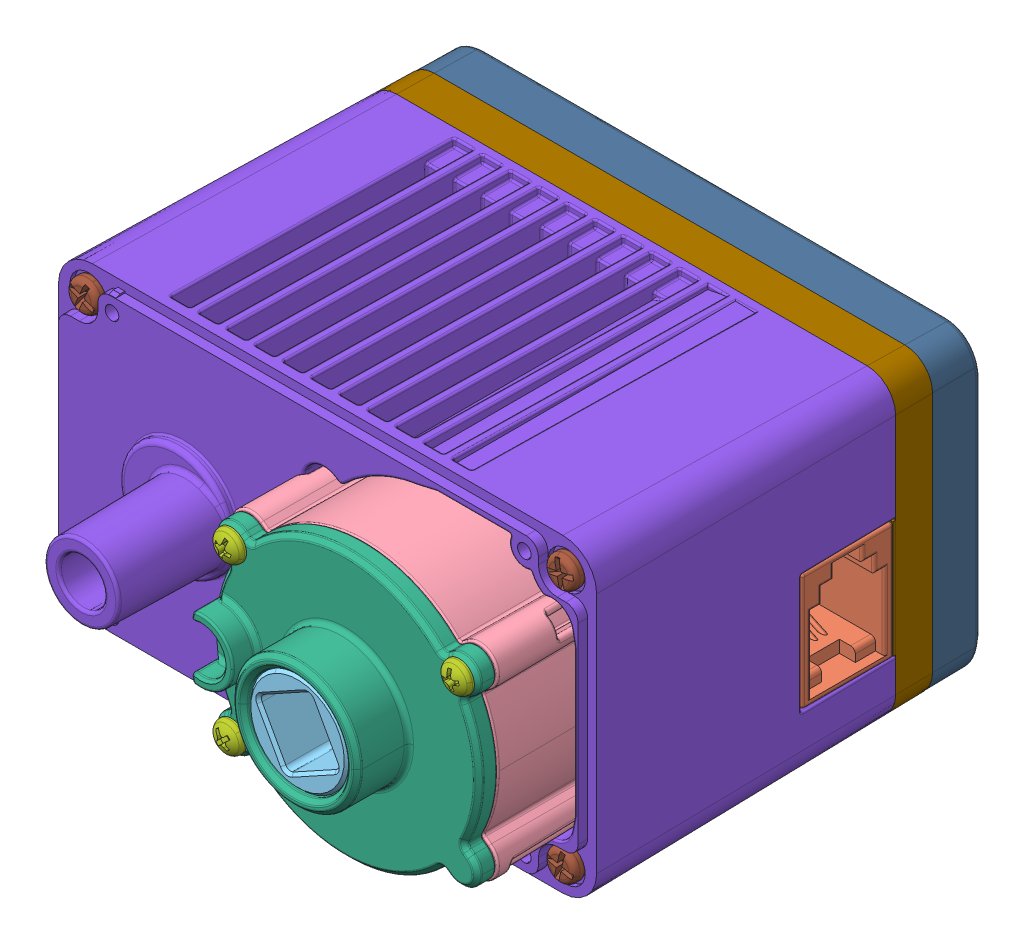
SolidWorks assembly V5 Smart Motor (276-4840) no cap 3, configuration Default. Lengths in mm.
Overall size (59.01 35.33 59.91).
20 component instances, 12 part files, 0 mates.
Components (placement in the parent):
- V5 Smart Motor (276-4840).step-1: V5 Smart Motor (276-4840).step [Default] at origin size (59.01 35.33 59.91)
  - 276-4840-900 Rev6_Instruction.step-1: 276-4840-900 Rev6_Instruction.step [Default] at (-14.3 0 -17.2) size (52.79 15.94 38.15)
    - 276-4840-901 Rev6.step-1: 276-4840-901 Rev6.step [Default] at (10.75 -10.05 17.8) x (-1 0 0) z (0 0 1) size (49.9 1.6 38.15)
    - 276-4840-902 Rev2.step-1: 276-4840-902 Rev2.step [Default] at (31.25 -9.25 6.2) x (0 0 -1) z (0 -1 0) size (10.35 11.39 15.94)
    - 276-4840-022 Rev4.step-1: 276-4840-022 Rev4.step [Default] at (31.25 -9.25 6.2) x (0 0 -1) z (1 0 0) size (10.26 9.1 5.51)
  - 276-4840-110 Rev10_Instruction.step-1: 276-4840-110 Rev10_Instruction.step [Default] at (12.7 0 14.7) size (35.33 35.33 31.1)
    - 276-4840-061 Rev7_Ring_Gear_Fixed01 .6 Rev3.step-1: 276-4840-061 Rev7_Ring_Gear_Fixed01 .6 Rev3.step [Default] at origin size (28.79 28.39 24.6)
    - 276-4840-018 Rev6.step-1: 276-4840-018 Rev6.step [Default] at (0 0 6.7) x (-0.483174 0.875524 0) z (0 0 1) size (26 26 12.3)
    - 276-4840-059 Rev2.step-1: 276-4840-059 Rev2.step [Default] at (0 0 10.3) size (28.4 28.4 8.5)
    - 276-4840-062 Rev1.step-1: 276-4840-062 Rev1.step [Default] at (-12.1353 8.8168 12.3) x (0.956835 -0.290632 0) z (-0.290632 -0.956835 0) size (3.2 6.56 3.2)
    - 276-4840-062 Rev1.step-2: 276-4840-062 Rev1.step [Default] at (12.1353 8.8168 12.3) x (0.978427 0.206591 0) z (0.206591 -0.978427 0) size (3.2 6.56 3.2)
    - 276-4840-062 Rev1.step-3: 276-4840-062 Rev1.step [Default] at (-12.1353 -8.8168 12.3) x (0.72563 0.688086 0) z (0.688086 -0.72563 0) size (3.2 6.56 3.2)
  - 276-4840-001 Rev38.step-1: 276-4840-001 Rev38.step [Default] at origin size (57.3 33 46.9)
  - 276-4840-005 Rev27.step-1: 276-4840-005 Rev27.step [Default] at (0 0 -17.95) size (56.17 31.87 12.9)
  - 276-4840-004 Rev16.step-1: 276-4840-004 Rev16.step [Default] at (0 0 -19.2) size (56.01 31.71 9.21)
  - 276-4840-009 Rev3.step-1: 276-4840-009 Rev3.step [Default] at (25.45 13.5 15.7) x (0.19987 -0.979823 0) z (-0.979823 -0.19987 0) size (3.4 41.31 4.34)
  - 276-4840-009 Rev3.step-2: 276-4840-009 Rev3.step [Default] at (-25.45 -13.5 15.7) x (-0.998855 0.047836 0) z (0.047836 0.998855 0) size (3.4 41.31 4.34)
  - 276-4840-009 Rev3.step-3: 276-4840-009 Rev3.step [Default] at (25.45 -13.5 15.7) x (-0.975374 0.220559 0) z (0.220559 0.975374 0) size (3.4 41.31 4.34)
  - 276-4840-009 Rev3.step-4: 276-4840-009 Rev3.step [Default] at (-25.45 13.5 15.7) x (-0.922256 0.38658 0) z (0.38658 0.922256 0) size (3.4 41.31 4.34)
  - 276-4840-025 Rev19.step-1: 276-4840-025 Rev19.step [Default] at (12.7 0 -22.63) x (-0.993315 0.115437 0) z (0 0 1) size (14.82 14.83 35.18)
